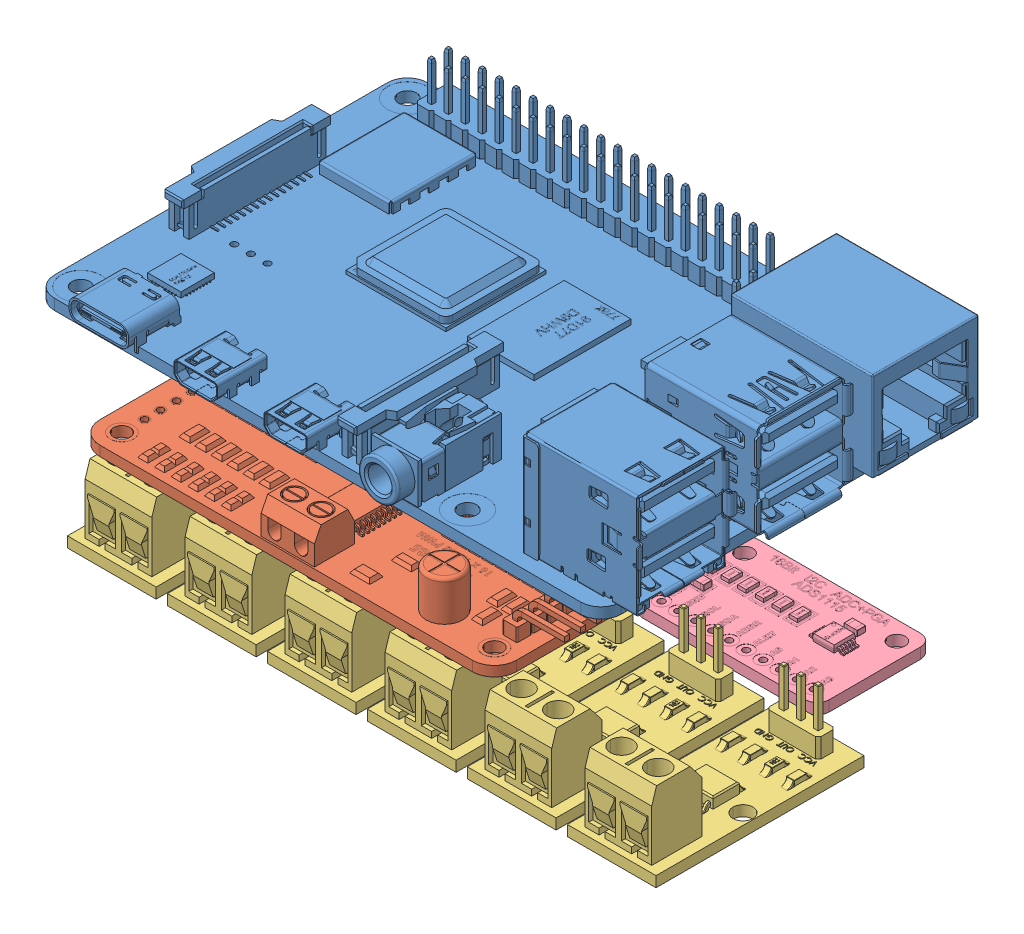
SolidWorks assembly ASM-Test, configuration По умолчанию. Lengths in mm.
Overall size (89.73 54.6 59.57).
10 component instances, 4 part files, 2 mates.
Components (placement in the parent):
- Raspberry Pi 4 Model B-1: Raspberry Pi 4 Model B [По умолчанию] at origin size (88.99 19.91 58.4)
- 12Channel PWM-1: 12Channel PWM [Default] at (-4.8787 -16.5453 15.1375) x (0 0 1) z (-1 0 0) size (25.4 7.55 66.7)
- 12Channel PWM-2: 12Channel PWM [Default] at (-4.8787 -16.5453 -14.013) x (0 0 1) z (-1 0 0) size (25.4 7.55 66.7)
- ACS712.step-1: ACS712.step [По умолчанию] at (-36.588 -36.3963 6.6868) x (0 0 1) z (-1 0 0) size (31.19 12.78 13.3)
- ACS712.step-2: ACS712.step [По умолчанию] at (-21.588 -36.3963 6.6868) x (0 0 1) z (-1 0 0) size (31.19 12.78 13.3)
- ACS712.step-3: ACS712.step [По умолчанию] at (-6.588 -36.3963 6.6868) x (0 0 1) z (-1 0 0) size (31.19 12.78 13.3)
- ACS712.step-4: ACS712.step [По умолчанию] at (8.412 -36.3963 6.6868) x (0 0 1) z (-1 0 0) size (31.19 12.78 13.3)
- ACS712.step-5: ACS712.step [По умолчанию] at (23.412 -36.3963 6.6868) x (0 0 1) z (-1 0 0) size (31.19 12.78 13.3)
- ACS712.step-6: ACS712.step [По умолчанию] at (38.412 -36.3963 6.6868) x (0 0 1) z (-1 0 0) size (31.19 12.78 13.3)
- 16Bit I2C ADC+PGA - ADS1115-1: 16Bit I2C ADC+PGA - ADS1115 [По умолчанию] at (21.1028 -36.5364 -20.5349) x (1 0 0) z (0 1 0) size (27.94 17.27 2.74)
Mates (geometry in assembly coordinates):
- Совпадение1: coincident aligned: plane of 12Channel PWM-1 through (23.0713 -15.0453 24.5375) normal (0 1 0); plane of 12Channel PWM-2 through (23.0713 -15.0453 -4.613) normal (0 1 0)
- Совпадение2: coincident aligned: plane of 12Channel PWM-1 through (-36.1287 -15.0453 5.7375) normal (-1 0 0); plane of 12Channel PWM-2 through (-36.1287 -15.0453 -23.413) normal (-1 0 0)
